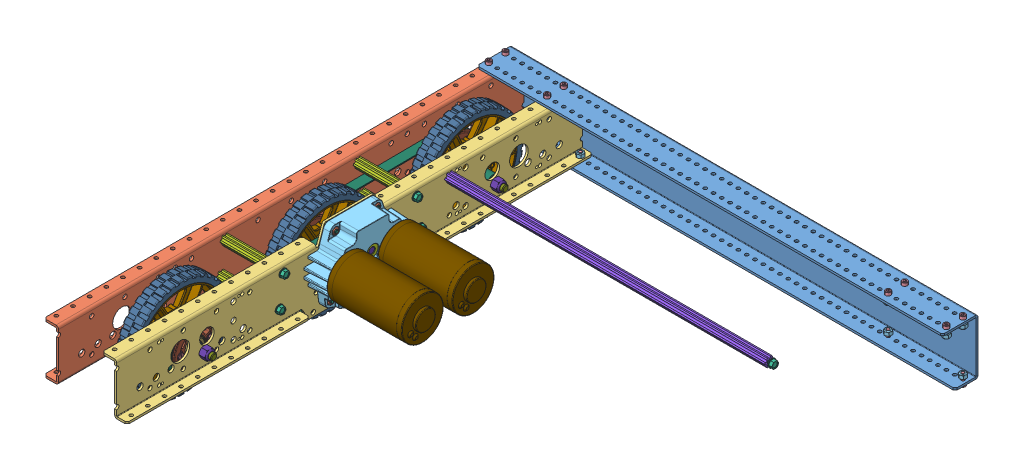
SolidWorks assembly AM14U4 Square Half, configuration Default. Lengths in mm.
Overall size (712.3 208.25 715.14).
150 component instances, 36 part files, 32 mates.
Components (placement in the parent):
- AM14U4 Square Frame Half-1: AM14U4 Square Frame Half [Default] at (318.96 74.5321 -359.8105) size (712.3 116.33 715.14)
  - am-xxxx AM14U4 End Plate Square-1: am-xxxx AM14U4 End Plate Square [Default] at (-787.4 -81.407 -3.175) x (1 0 0) z (0 -1 0) size (711.2 53.98 84.58)
  - am-xxxx AM14U4 Outside Plate Square-1: am-xxxx AM14U4 Outside Plate Square [DefaultSM-FLAT-PATTERN] at (-692.15 -77.216 762.762) x (0 0 -1) z (0 -1 0) size (711.2 22.23 77.72)
  - am-xxxx AM14U4 Inside Plate Square-1: am-xxxx AM14U4 Inside Plate Square [Default] at (-603.25 -77.216 762.762) x (0 0 -1) z (0 -1 0) size (711.2 38.1 116.33)
  - am-1002 and am-1042 10-32 x 0500 and Nylock Nut Assembly-2: am-1002 and am-1042 10-32 x 0500 and Nylock Nut Assembly [Default] at (-708.3821 -6.6363 35.2132) x (0 -1 0) z (0 0 1) size (17.53 13.8 13)
    - 10-32x0500_shcs-1: 10-32x0500_shcs [HX-SHCS 0.19-32x1.375x1-C] at (-11.4623 3.5321 3.6488) size (17.53 7.94 7.94)
    - 10-32 Nylock Nut 1-1: 10-32 Nylock Nut 1 [90631A411] at (-0.0323 3.5321 3.6488) x (0 0.381849 -0.924225) z (0 -0.924225 -0.381849) size (9.53 6.11 11)
  - am-1002 and am-1042 10-32 x 0500 and Nylock Nut Assembly-3: am-1002 and am-1042 10-32 x 0500 and Nylock Nut Assembly [Default] at (-708.3821 -6.6363 9.8132) x (0 -1 0) z (0 0 1) size (17.53 13.8 13)
    - 10-32x0500_shcs-1: 10-32x0500_shcs [HX-SHCS 0.19-32x1.375x1-C] at (-11.4623 3.5321 3.6488) size (17.53 7.94 7.94)
    - 10-32 Nylock Nut 1-1: 10-32 Nylock Nut 1 [90631A411] at (-0.0323 3.5321 3.6488) x (0 0.381849 -0.924225) z (0 -0.924225 -0.381849) size (9.53 6.11 11)
  - am-1002 and am-1042 10-32 x 0500 and Nylock Nut Assembly-7: am-1002 and am-1042 10-32 x 0500 and Nylock Nut Assembly [Default] at (-701.3179 -77.9457 9.8132) x (0 1 0) z (0 0 1) size (17.53 13.8 13)
    - 10-32x0500_shcs-1: 10-32x0500_shcs [HX-SHCS 0.19-32x1.375x1-C] at (-11.4623 3.5321 3.6488) size (17.53 7.94 7.94)
    - 10-32 Nylock Nut 1-1: 10-32 Nylock Nut 1 [90631A411] at (-0.0323 3.5321 3.6488) x (0 0.381849 -0.924225) z (0 -0.924225 -0.381849) size (9.53 6.11 11)
  - am-1002 and am-1042 10-32 x 0500 and Nylock Nut Assembly-8: am-1002 and am-1042 10-32 x 0500 and Nylock Nut Assembly [Default] at (-9.8821 -6.6363 9.8132) x (0 -1 0) z (0 0 1) size (17.53 13.8 13)
    - 10-32x0500_shcs-1: 10-32x0500_shcs [HX-SHCS 0.19-32x1.375x1-C] at (-11.4623 3.5321 3.6488) size (17.53 7.94 7.94)
    - 10-32 Nylock Nut 1-1: 10-32 Nylock Nut 1 [90631A411] at (-0.0323 3.5321 3.6488) x (0 0.381849 -0.924225) z (0 -0.924225 -0.381849) size (9.53 6.11 11)
  - am-1002 and am-1042 10-32 x 0500 and Nylock Nut Assembly-9: am-1002 and am-1042 10-32 x 0500 and Nylock Nut Assembly [Default] at (-9.8821 -6.6363 35.2132) x (0 -1 0) z (0 0 1) size (17.53 13.8 13)
    - 10-32x0500_shcs-1: 10-32x0500_shcs [HX-SHCS 0.19-32x1.375x1-C] at (-11.4623 3.5321 3.6488) size (17.53 7.94 7.94)
    - 10-32 Nylock Nut 1-1: 10-32 Nylock Nut 1 [90631A411] at (-0.0323 3.5321 3.6488) x (0 0.381849 -0.924225) z (0 -0.924225 -0.381849) size (9.53 6.11 11)
  - am-1002 and am-1042 10-32 x 0500 and Nylock Nut Assembly-10: am-1002 and am-1042 10-32 x 0500 and Nylock Nut Assembly [Default] at (-2.8179 -77.9457 9.8132) x (0 1 0) z (0 0 1) size (17.53 13.8 13)
    - 10-32x0500_shcs-1: 10-32x0500_shcs [HX-SHCS 0.19-32x1.375x1-C] at (-11.4623 3.5321 3.6488) size (17.53 7.94 7.94)
    - 10-32 Nylock Nut 1-1: 10-32 Nylock Nut 1 [90631A411] at (-0.0323 3.5321 3.6488) x (0 0.381849 -0.924225) z (0 -0.924225 -0.381849) size (9.53 6.11 11)
  - am-1002 and am-1042 10-32 x 0500 and Nylock Nut Assembly-11: am-1002 and am-1042 10-32 x 0500 and Nylock Nut Assembly [Default] at (-117.1179 -77.9457 9.8132) x (0 1 0) z (0 0 1) size (17.53 13.8 13)
    - 10-32x0500_shcs-1: 10-32x0500_shcs [HX-SHCS 0.19-32x1.375x1-C] at (-11.4623 3.5321 3.6488) size (17.53 7.94 7.94)
    - 10-32 Nylock Nut 1-1: 10-32 Nylock Nut 1 [90631A411] at (-0.0323 3.5321 3.6488) x (0 0.381849 -0.924225) z (0 -0.924225 -0.381849) size (9.53 6.11 11)
  - am-1002 and am-1042 10-32 x 0500 and Nylock Nut Assembly-12: am-1002 and am-1042 10-32 x 0500 and Nylock Nut Assembly [Default] at (-98.7821 -6.6363 35.2132) x (0 -1 0) z (0 0 1) size (17.53 13.8 13)
    - 10-32x0500_shcs-1: 10-32x0500_shcs [HX-SHCS 0.19-32x1.375x1-C] at (-11.4623 3.5321 3.6488) size (17.53 7.94 7.94)
    - 10-32 Nylock Nut 1-1: 10-32 Nylock Nut 1 [90631A411] at (-0.0323 3.5321 3.6488) x (0 0.381849 -0.924225) z (0 -0.924225 -0.381849) size (9.53 6.11 11)
  - am-1002 and am-1042 10-32 x 0500 and Nylock Nut Assembly-13: am-1002 and am-1042 10-32 x 0500 and Nylock Nut Assembly [Default] at (-98.7821 -6.6363 9.8132) x (0 -1 0) z (0 0 1) size (17.53 13.8 13)
    - 10-32x0500_shcs-1: 10-32x0500_shcs [HX-SHCS 0.19-32x1.375x1-C] at (-11.4623 3.5321 3.6488) size (17.53 7.94 7.94)
    - 10-32 Nylock Nut 1-1: 10-32 Nylock Nut 1 [90631A411] at (-0.0323 3.5321 3.6488) x (0 0.381849 -0.924225) z (0 -0.924225 -0.381849) size (9.53 6.11 11)
  - FHTS 0.25-20-0.75-1: FHTS 0.25-20-0.75 [FHTS 0.25-20-G-0.75-C] at (-692.15 -59.6687 248.8365) size (24.64 12.19 12.19)
  - FHTS 0.25-20-0.75-2: FHTS 0.25-20-0.75 [FHTS 0.25-20-G-0.75-C] at (-692.15 -14.986 254.762) size (24.64 12.19 12.19)
  - FHTS 0.25-20-0.75-3: FHTS 0.25-20-0.75 [FHTS 0.25-20-G-0.75-C] at (-692.15 -14.986 457.962) size (24.64 12.19 12.19)
  - FHTS 0.25-20-0.75-4: FHTS 0.25-20-0.75 [FHTS 0.25-20-G-0.75-C] at (-692.15 -59.6687 463.8875) size (24.64 12.19 12.19)
  - FHTS 0.25-20-0.75-5: FHTS 0.25-20-0.75 [FHTS 0.25-20-G-0.75-C] at (-600.075 -14.986 457.962) x (-1 0 0) z (0 0.924225 0.381849) size (24.64 12.19 12.19)
  - FHTS 0.25-20-0.75-6: FHTS 0.25-20-0.75 [FHTS 0.25-20-G-0.75-C] at (-600.075 -59.6687 463.8875) x (-1 0 0) z (0 0.924225 0.381849) size (24.64 12.19 12.19)
  - FHTS 0.25-20-0.75-7: FHTS 0.25-20-0.75 [FHTS 0.25-20-G-0.75-C] at (-600.075 -14.986 254.762) x (-1 0 0) z (0 0.924225 0.381849) size (24.64 12.19 12.19)
  - FHTS 0.25-20-0.75-8: FHTS 0.25-20-0.75 [FHTS 0.25-20-G-0.75-C] at (-600.075 -59.6687 248.8365) x (-1 0 0) z (0 0.924225 0.381849) size (24.64 12.19 12.19)
  - 3.375in Churro-1: 3.375in Churro [Default] at (-603.25 -14.986 254.762) x (0 0 1) z (-1 0 0) size (14.66 12.7 85.72)
  - 3.375in Churro-2: 3.375in Churro [Default] at (-606.425 -59.6687 248.8365) x (0 0 1) z (-1 0 0) size (14.66 12.7 85.72)
  - 3.375in Churro-3: 3.375in Churro [Default] at (-603.25 -14.986 457.962) x (0 0 1) z (-1 0 0) size (14.66 12.7 85.72)
  - 3.375in Churro-4: 3.375in Churro [Default] at (-603.25 -59.6687 463.8875) x (0 0 1) z (-1 0 0) size (14.66 12.7 85.72)
  - am-1002 and am-1042 10-32 x 0500 and Nylock Nut Assembly-14: am-1002 and am-1042 10-32 x 0500 and Nylock Nut Assembly [Default] at (-619.4821 -6.6363 9.8132) x (0 -1 0) z (0 0 1) size (17.53 13.8 13)
    - 10-32x0500_shcs-1: 10-32x0500_shcs [HX-SHCS 0.19-32x1.375x1-C] at (-11.4623 3.5321 3.6488) size (17.53 7.94 7.94)
    - 10-32 Nylock Nut 1-1: 10-32 Nylock Nut 1 [90631A411] at (-0.0323 3.5321 3.6488) x (0 0.381849 -0.924225) z (0 -0.924225 -0.381849) size (9.53 6.11 11)
  - am-1002 and am-1042 10-32 x 0500 and Nylock Nut Assembly-15: am-1002 and am-1042 10-32 x 0500 and Nylock Nut Assembly [Default] at (-619.4821 -6.6363 35.2132) x (0 -1 0) z (0 0 1) size (17.53 13.8 13)
    - 10-32x0500_shcs-1: 10-32x0500_shcs [HX-SHCS 0.19-32x1.375x1-C] at (-11.4623 3.5321 3.6488) size (17.53 7.94 7.94)
    - 10-32 Nylock Nut 1-1: 10-32 Nylock Nut 1 [90631A411] at (-0.0323 3.5321 3.6488) x (0 0.381849 -0.924225) z (0 -0.924225 -0.381849) size (9.53 6.11 11)
  - am-1002 and am-1042 10-32 x 0500 and Nylock Nut Assembly-16: am-1002 and am-1042 10-32 x 0500 and Nylock Nut Assembly [Default] at (-587.0179 -77.9457 9.8132) x (0 1 0) z (0 0 1) size (17.53 13.8 13)
    - 10-32x0500_shcs-1: 10-32x0500_shcs [HX-SHCS 0.19-32x1.375x1-C] at (-11.4623 3.5321 3.6488) size (17.53 7.94 7.94)
    - 10-32 Nylock Nut 1-1: 10-32 Nylock Nut 1 [90631A411] at (-0.0323 3.5321 3.6488) x (0 0.381849 -0.924225) z (0 -0.924225 -0.381849) size (9.53 6.11 11)
  - 19.25in Churro-1: 19.25in Churro [Default] at (-355.6 -14.986 203.962) x (0 0 1) z (-1 0 0) size (14.66 12.7 488.95)
  - FHTS 0.25-20-0.75-9: FHTS 0.25-20-0.75 [FHTS 0.25-20-G-0.75-C] at (-603.25 -14.986 203.962) size (24.64 12.19 12.19)
  - FHTS 0.25-20-0.75-10: FHTS 0.25-20-0.75 [FHTS 0.25-20-G-0.75-C] at (-107.95 -14.986 203.962) x (-1 0 0) z (0 -0.866025 -0.5) size (24.64 12.19 12.19)
- 6 HiGrip with bearings, pulleys and spacers-1: 6 HiGrip with bearings, pulleys and spacers [Default] at (-295.3634 -45.2429 -85.8734) x (-1 0 0) z (0 -0.111601 -0.993753) size (85.56 152.4 152.4)
  - 6 HiGrip Asm Rev II-1: 6 HiGrip Asm Rev II [Default] at (83.7987 67.439 110.9939) size (35.05 152.4 152.4)
    - 6 wheel Rev 4-1: 6 wheel Rev 4 [Default] at (-52.6446 9.4231 21.378) size (35.05 132.08 132.08)
    - 6 wheel tread II-1: 6 wheel tread II [Default] at (-65.3446 9.4231 21.378) x (0 0 -1) z (1 0 0) size (152.4 152.4 25.58)
  - 42 tooth HTD Pulley half 2014-1: 42 tooth HTD Pulley half 2014 [Default] at (47.6006 76.862 132.3719) x (1 0 0) z (0 -0.5 0.866025) size (13 74.23 74.23)
  - 42 tooth HTD Pulley half 2014-2: 42 tooth HTD Pulley half 2014 [Default] at (64.263 76.862 132.3719) x (-1 0 0) z (0 -0.499927 0.866067) size (13 74.23 74.23)
  - 1614Z Bearing-1: 1614Z Bearing [Default] at (62.612 76.862 132.3719) x (0 -0.157148 -0.987575) z (-1 0 0) size (28.57 28.57 9.53)
  - 10-24 Hex Washer Rolling x 1.25-1: 10-24 Hex Washer Rolling x 1.25 [93882A213] at (63.247 76.8605 108.5602) x (0 0 -1) z (1 0 0) size (10.52 10.52 35.59)
  - 10-24 Hex Washer Rolling x 1.25-2: 10-24 Hex Washer Rolling x 1.25 [93882A213] at (63.247 97.4833 120.4656) x (0 0 -1) z (1 0 0) size (10.52 10.52 35.59)
  - 10-24 Hex Washer Rolling x 1.25-3: 10-24 Hex Washer Rolling x 1.25 [93882A213] at (63.247 56.2398 144.2799) x (0 0 -1) z (1 0 0) size (10.52 10.52 35.59)
  - 10-24 Hex Washer Rolling x 1.25-4: 10-24 Hex Washer Rolling x 1.25 [93882A213] at (63.247 76.8625 156.1852) x (0 -0.95788 -0.287168) z (1 0 0) size (10.52 10.52 35.59)
  - 10-24 Hex Washer Rolling x 1.25-5: 10-24 Hex Washer Rolling x 1.25 [93882A213] at (63.247 97.4843 144.2781) x (0 -0.868976 0.494854) z (1 0 0) size (10.52 10.52 35.59)
  - 10-24 Hex Washer Rolling x 1.25-6: 10-24 Hex Washer Rolling x 1.25 [93882A213] at (63.247 56.2388 120.4674) x (0 -0.977348 -0.211637) z (1 0 0) size (10.52 10.52 35.59)
  - am-1306 spacer 0280 WashersUSA 13RS052001-1: am-1306 spacer 0280 WashersUSA 13RS052001 [Default] at (74.4865 76.862 132.3719) x (0 -0.35357 0.935408) z (-1 0 0) size (13.16 13.16 7.11)
  - 1614Z Bearing-2: 1614Z Bearing [Default] at (15.2791 76.862 132.3719) x (0 0.155433 -0.987846) z (-1 0 0) size (28.57 28.57 9.53)
  - am-1307 850 long 380 id-1: am-1307 850 long 380 id [Default] at (10.5166 76.862 132.3719) x (0 0.971418 -0.237374) z (0 0.237374 0.971418) size (19.05 21.59 19.05)
- 6 HiGrip with bearings, pulleys and spacers-2: 6 HiGrip with bearings, pulleys and spacers [Default] at (-358.7765 -60.4959 86.7273) size (85.56 152.4 152.4)
  - 6 HiGrip Asm Rev II-1: 6 HiGrip Asm Rev II [Default] at (83.7987 67.439 110.9939) size (35.05 152.4 152.4)
    - 6 wheel Rev 4-1: 6 wheel Rev 4 [Default] at (-52.6446 9.4231 21.378) size (35.05 132.08 132.08)
    - 6 wheel tread II-1: 6 wheel tread II [Default] at (-65.3446 9.4231 21.378) x (0 0 -1) z (1 0 0) size (152.4 152.4 25.58)
  - 42 tooth HTD Pulley half 2014-1: 42 tooth HTD Pulley half 2014 [Default] at (47.6006 76.862 132.3719) x (1 0 0) z (0 -0.5 0.866025) size (13 74.23 74.23)
  - 42 tooth HTD Pulley half 2014-2: 42 tooth HTD Pulley half 2014 [Default] at (64.263 76.862 132.3719) x (-1 0 0) z (0 -0.499927 0.866067) size (13 74.23 74.23)
  - 1614Z Bearing-1: 1614Z Bearing [Default] at (62.612 76.862 132.3719) x (0 -0.157148 -0.987575) z (-1 0 0) size (28.57 28.57 9.53)
  - 10-24 Hex Washer Rolling x 1.25-1: 10-24 Hex Washer Rolling x 1.25 [93882A213] at (63.247 76.8605 108.5602) x (0 0 -1) z (1 0 0) size (10.52 10.52 35.59)
  - 10-24 Hex Washer Rolling x 1.25-2: 10-24 Hex Washer Rolling x 1.25 [93882A213] at (63.247 97.4833 120.4656) x (0 0 -1) z (1 0 0) size (10.52 10.52 35.59)
  - 10-24 Hex Washer Rolling x 1.25-3: 10-24 Hex Washer Rolling x 1.25 [93882A213] at (63.247 56.2398 144.2799) x (0 0 -1) z (1 0 0) size (10.52 10.52 35.59)
  - 10-24 Hex Washer Rolling x 1.25-4: 10-24 Hex Washer Rolling x 1.25 [93882A213] at (63.247 76.8625 156.1852) x (0 -0.95788 -0.287168) z (1 0 0) size (10.52 10.52 35.59)
  - 10-24 Hex Washer Rolling x 1.25-5: 10-24 Hex Washer Rolling x 1.25 [93882A213] at (63.247 97.4843 144.2781) x (0 -0.868976 0.494854) z (1 0 0) size (10.52 10.52 35.59)
  - 10-24 Hex Washer Rolling x 1.25-6: 10-24 Hex Washer Rolling x 1.25 [93882A213] at (63.247 56.2388 120.4674) x (0 -0.977348 -0.211637) z (1 0 0) size (10.52 10.52 35.59)
  - am-1306 spacer 0280 WashersUSA 13RS052001-1: am-1306 spacer 0280 WashersUSA 13RS052001 [Default] at (74.4865 76.862 132.3719) x (0 -0.35357 0.935408) z (-1 0 0) size (13.16 13.16 7.11)
  - 1614Z Bearing-2: 1614Z Bearing [Default] at (15.2791 76.862 132.3719) x (0 0.155433 -0.987846) z (-1 0 0) size (28.57 28.57 9.53)
  - am-1307 850 long 380 id-1: am-1307 850 long 380 id [Default] at (10.5166 76.862 132.3719) x (0 0.971418 -0.237374) z (0 0.237374 0.971418) size (19.05 21.59 19.05)
- FR8ZZ Hex Bearing-1: FR8ZZ Hex Bearing [Default] at (-376.4183 14.5881 -3.4485) x (0 0 -1) z (1 0 0) size (31.12 31.12 7.93)
- am-2598_107 2016 KOP Toughbox Mini-1: am-2598_107 2016 KOP Toughbox Mini [Default] at (-331.6566 4.5181 87.6522) x (0 0.001296 0.999999) z (-1 0 0) size (140.05 121.81 142.29)
  - Toughbox d07-1: Toughbox d07 [Default] at (-88.5589 93.4503 -52.3959) x (-0.336928 0.94153 0) z (0.94153 0.336928 0) size (11 38.23 9.52)
  - Toughbox d05-1: Toughbox d05 [Default] at (-91.0349 50.9043 -67.5597) x (-0.336928 0.94153 0) z (0 0 -1) size (65.97 66.04 10.16)
  - FR6ZZ Bearing-1: FR6ZZ Bearing [Default] at (-96.247 60.278 -52.5991) x (-0.893862 0.448342 0) z (0 0 1) size (24.69 24.69 7.16)
  - 10-32 Nylock Nut-1: 10-32 Nylock Nut [Default] at (-129.8464 -8.0737 -56.3837) x (0.501678 0.865055 0) z (0 0 -1) size (10.18 11.01 7.1)
  - 10-32 Nylock Nut-2: 10-32 Nylock Nut [Default] at (-59.2462 80.7349 -56.3837) x (0.999999 -0.001296 0) z (0 0 -1) size (10.18 11.01 7.1)
  - 10-32 Nylock Nut-3: 10-32 Nylock Nut [Default] at (-122.7461 80.8172 -56.3837) x (0.500567 0.865698 0) z (0 0 -1) size (10.18 11.01 7.1)
  - 10-32 Nylock Nut-4: 10-32 Nylock Nut [Default] at (-52.3764 -8.1741 -56.3837) x (-0.501678 -0.865055 0) z (0 0 -1) size (10.18 11.01 7.1)
  - 5-16 washer-1: 5-16 washer [Default] at (-52.3162 38.3079 -77.7705) x (0.38418 -0.923258 0) z (0 0 -1) size (17.53 17.53 1.47)
  - 5-16 washer-2: 5-16 washer [Default] at (-52.3162 38.3079 -76.2973) x (0.897267 -0.441488 0) z (0 0 -1) size (17.53 17.53 1.47)
  - 5-16 washer-3: 5-16 washer [Default] at (-129.7861 38.4083 -77.7705) x (-0.990116 0.140253 0) z (0 0 1) size (17.53 17.53 1.47)
  - 5-16 washer-4: 5-16 washer [Default] at (-129.7861 38.4083 -79.2437) x (-0.681761 0.731575 0) z (0 0 1) size (17.53 17.53 1.47)
  - Toughbox d09-1: Toughbox d09 [Default] at (-52.3162 38.3079 -63.5973) x (0.910249 -0.414061 0) z (0 0 -1) size (20.03 20.32 12.7)
  - Toughbox d09-2: Toughbox d09 [Default] at (-129.7861 38.4083 -63.5973) x (0.075368 -0.997156 0) z (0 0 -1) size (20.03 20.32 12.7)
  - TM Housing-1: TM Housing [Default] at (-91.0876 10.1882 -86.3557) x (0.999999 -0.001296 0) z (0 0 1) size (139.9 118.55 41.54)
  - SHCS 10-32 x 0.625-1: SHCS 10-32 x 0.625 [Default] at (-52.2832 63.7078 -74.4685) x (-0.564778 -0.825243 0) z (-0.825243 0.564778 0) size (7.82 20.65 7.82)
  - SHCS 10-32 x 0.625-2: SHCS 10-32 x 0.625 [Default] at (-122.7461 80.8172 -42.5915) x (0.507484 -0.861661 0) z (-0.861661 -0.507484 0) size (7.82 20.65 7.82)
  - SHCS 10-32 x 0.625-3: SHCS 10-32 x 0.625 [Default] at (-52.3764 -8.1741 -42.5915) x (0.507484 -0.861661 0) z (-0.861661 -0.507484 0) size (7.82 20.65 7.82)
  - SHCS 10-32 x 0.625-4: SHCS 10-32 x 0.625 [Default] at (-129.8464 -8.0737 -42.5915) x (0.507484 -0.861661 0) z (-0.861661 -0.507484 0) size (7.82 20.65 7.82)
  - SHCS 10-32 x 0.625-5: SHCS 10-32 x 0.625 [Default] at (-59.2462 80.7349 -42.5915) x (0.740711 -0.671824 0) z (-0.671824 -0.740711 0) size (7.82 20.65 7.82)
  - SHCS 10-32 x 0.625-6: SHCS 10-32 x 0.625 [Default] at (-52.3491 12.9079 -74.4685) x (-0.564778 -0.825243 0) z (-0.825243 0.564778 0) size (7.82 20.65 7.82)
  - SHCS 10-32 x 0.625-7: SHCS 10-32 x 0.625 [Default] at (-129.7532 63.8083 -74.4685) x (-0.966277 -0.257503 0) z (-0.257503 0.966277 0) size (7.82 20.65 7.82)
  - SHCS 10-32 x 0.625-8: SHCS 10-32 x 0.625 [Default] at (-129.819 13.0083 -74.4685) x (-0.99652 0.083357 0) z (0.083357 0.99652 0) size (7.82 20.65 7.82)
  - R6ZZ Bearing-3: R6ZZ Bearing [Default] at (-91.0349 50.9043 -84.8317) x (0.958138 -0.286306 0) z (0 0 1) size (22.23 22.23 7.11)
  - R6ZZ Bearing-4: R6ZZ Bearing [Default] at (-91.0876 10.1882 -84.8317) x (-0.328282 -0.94458 0) z (0 0 1) size (22.23 22.23 7.11)
  - 8mm spring clip-1: 8mm spring clip [Default] at (-129.7861 38.4083 -63.5973) x (0 0 1) z (-1 0 0) size (1.09 14.83 14.83)
  - 8mm spring clip-2: 8mm spring clip [Default] at (-52.3162 38.3079 -63.5973) x (0 0 1) z (-1 0 0) size (1.09 14.83 14.83)
  - 500 E-klip-1: 500 E-klip [Default] at (-91.0876 10.1882 -64.4355) x (0.996411 -0.084651 0) z (0 0 1) size (19.07 20.96 1.27)
  - FR8ZZ Hex Bearing-1: FR8ZZ Hex Bearing [Default] at (-91.0876 10.1882 -44.6717) x (-0.5 0.866025 0) z (0 0 -1) size (31.12 31.12 7.93)
  - 16t 20dp 375h with teeth-1: 16t 20dp 375h with teeth [Default] at (-91.0349 50.9043 -67.5597) x (0 0 1) z (-0.983853 0.178977 0) size (15.19 22.57 22.57)
  - 48t 20dp 500h with teeth-1: 48t 20dp 500h with teeth [Default] at (-91.0876 10.1882 -63.1655) x (0 0 1) z (-1 0 0) size (10.21 63.42 63.42)
  - TB Output Shaft Hex L-Base 2-1: TB Output Shaft Hex L-Base 2 [Default] at (-52.7805 -6.4809 -52.3197) x (1 0 0) z (0 -1 0) size (14.66 142.29 12.7)
- 6 HiGrip with hub and double pulley-1: 6 HiGrip with hub and double pulley [Default] at (-295.2897 167.6569 -3.2676) x (-1 0 0) z (0 -0.865376 0.501122) size (81.42 152.4 152.4)
  - 6 HiGrip Asm Rev II-1: 6 HiGrip Asm Rev II [Default] at (83.7987 67.439 110.9939) size (35.05 152.4 152.4)
    - 6 wheel Rev 4-1: 6 wheel Rev 4 [Default] at (-52.6446 9.4231 21.378) size (35.05 132.08 132.08)
    - 6 wheel tread II-1: 6 wheel tread II [Default] at (-65.3446 9.4231 21.378) x (0 0 -1) z (1 0 0) size (152.4 152.4 25.58)
  - 42 tooth HTD Pulley half 2014-1: 42 tooth HTD Pulley half 2014 [Default] at (47.6006 76.862 132.3719) x (1 0 0) z (0 -0.5 0.866025) size (13 74.23 74.23)
  - 42 tooth HTD Pulley half 2014-2: 42 tooth HTD Pulley half 2014 [Default] at (64.263 76.862 132.3719) x (-1 0 0) z (0 -0.499927 0.866067) size (13 74.23 74.23)
  - 10-24 Hex Washer Rolling x 1.25-1: 10-24 Hex Washer Rolling x 1.25 [93882A213] at (63.247 76.8605 108.5602) x (0 0 -1) z (1 0 0) size (10.52 10.52 35.59)
  - 10-24 Hex Washer Rolling x 1.25-2: 10-24 Hex Washer Rolling x 1.25 [93882A213] at (63.247 97.4833 120.4656) x (0 0 -1) z (1 0 0) size (10.52 10.52 35.59)
  - 10-24 Hex Washer Rolling x 1.25-3: 10-24 Hex Washer Rolling x 1.25 [93882A213] at (63.247 56.2398 144.2799) x (0 0 -1) z (1 0 0) size (10.52 10.52 35.59)
  - 10-24 Hex Washer Rolling x 1.25-4: 10-24 Hex Washer Rolling x 1.25 [93882A213] at (63.247 76.8625 156.1852) x (0 -0.95788 -0.287168) z (1 0 0) size (10.52 10.52 35.59)
  - 10-24 Hex Washer Rolling x 1.25-5: 10-24 Hex Washer Rolling x 1.25 [93882A213] at (63.247 97.4843 144.2781) x (0 -0.868976 0.494854) z (1 0 0) size (10.52 10.52 35.59)
  - 10-24 Hex Washer Rolling x 1.25-6: 10-24 Hex Washer Rolling x 1.25 [93882A213] at (63.247 56.2388 120.4674) x (0 -0.748729 -0.662876) z (1 0 0) size (10.52 10.52 35.59)
  - 42 tooth HTD Pulley half 2014-3: 42 tooth HTD Pulley half 2014 [Default] at (-1.9548 76.8628 132.3714) x (1 0 0) z (0 -1 -0.000063) size (13 74.23 74.23)
  - 42 tooth HTD Pulley half 2014-4: 42 tooth HTD Pulley half 2014 [Default] at (14.7076 76.8628 132.3714) x (-1 0 0) z (0 -1 0.000021) size (13 74.23 74.23)
  - 500EX Hex Hub-1: 500EX Hex Hub [Default] at (-8.3048 76.8628 132.3714) x (0 -0.866025 -0.5) z (0 -0.5 0.866025) size (55.37 25.4 51.33)
  - 10-24 Hex Washer Rolling x 1.25-7: 10-24 Hex Washer Rolling x 1.25 [93882A213] at (-5.2568 97.485 120.4652) x (0 0 1) z (-1 0 0) size (10.52 10.52 35.59)
  - 10-24 Hex Washer Rolling x 1.25-8: 10-24 Hex Washer Rolling x 1.25 [93882A213] at (-5.2568 76.8628 108.5589) x (0 0 1) z (-1 0 0) size (10.52 10.52 35.59)
  - 10-24 Hex Washer Rolling x 1.25-9: 10-24 Hex Washer Rolling x 1.25 [93882A213] at (-5.2568 56.2406 120.4652) x (0 0 1) z (-1 0 0) size (10.52 10.52 35.59)
  - 10-24 Hex Washer Rolling x 1.25-10: 10-24 Hex Washer Rolling x 1.25 [93882A213] at (-5.2568 97.485 144.2777) x (0 -0.99374 -0.111715) z (-1 0 0) size (10.52 10.52 35.59)
  - 10-24 Hex Washer Rolling x 1.25-11: 10-24 Hex Washer Rolling x 1.25 [93882A213] at (-5.2568 56.2406 144.2777) x (0 -0.138911 0.990305) z (-1 0 0) size (10.52 10.52 35.59)
  - 10-24 Hex Washer Rolling x 1.25-12: 10-24 Hex Washer Rolling x 1.25 [93882A213] at (-5.2568 76.8628 156.1839) x (0 -0.98811 -0.15375) z (-1 0 0) size (10.52 10.52 35.59)
  - am-1305 500 Hex Spacer-1: am-1305 500 Hex Spacer [Default] at (57.8495 76.862 132.3719) x (0 -0.866025 -0.5) z (0 -0.5 0.866025) size (28.55 14.48 28.55)
- 655-5M-15 v2-1: 655-5M-15 v2 [Default] at (-357.8903 14.5881 -3.4485) x (0 0.007989 -0.999968) z (0 -0.999968 -0.007989) size (295.63 15 73.08)
- 655-5M-15 v2-2: 655-5M-15 v2 [Default] at (-309.9973 14.5881 -3.4485) x (0 0.007989 0.999968) z (0 0.999968 -0.007989) size (295.63 15 73.08)
- 375-16 x 4.25 Hex Bolt-1: 375-16 x 4.25 Hex Bolt [HFBOLT 0.375-16x2.5x1-C] at (-379.3622 16.3661 -225.9962) size (114.12 16.48 14.27)
- 375-16 x 4.25 Hex Bolt-2: 375-16 x 4.25 Hex Bolt [HFBOLT 0.375-16x2.5x1-C] at (-379.3622 16.3661 219.0992) size (114.12 16.48 14.27)
- 3-8-16 NyLock Nut - Mcm 95615A140-1: 3-8-16 NyLock Nut - Mcm 95615A140 [95615A140] at (-281.115 16.3661 -225.9962) x (0 -1 0) z (0 0 1) size (14.29 12 16.5)
- 3-8-16 NyLock Nut - Mcm 95615A140-2: 3-8-16 NyLock Nut - Mcm 95615A140 [95615A140] at (-281.115 16.3661 219.0992) x (0 -1 0) z (0 0 1) size (14.29 12 16.5)
- CIM Motor SW-1: CIM Motor SW [Default] at (-226.251 78.3181 -151.4797) x (0 -1 0) z (-1 0 0) size (64.01 64.01 154.93)
- CIM Motor SW-2: CIM Motor SW [Default] at (-226.251 78.3181 -74.0097) x (0 -1 0) z (-1 0 0) size (64.01 64.01 154.93)
Mates (geometry in assembly coordinates):
- Coincident1: coincident: plane of AM14U4 Square Frame Half-1/am-xxxx AM14U4 Inside Plate Square-1 through (-284.29 67.1661 402.9515) normal (-1 0 0); plane of 6 HiGrip with bearings, pulleys and spacers-2/am-1306 spacer 0280 WashersUSA 13RS052001-1 through (-284.29 16.3661 219.0992) normal (1 0 0)
- Concentric1: concentric: circle of AM14U4 Square Frame Half-1/am-xxxx AM14U4 Inside Plate Square-1; cylinder of 6 HiGrip with bearings, pulleys and spacers-2/am-1306 spacer 0280 WashersUSA 13RS052001-1 through (-291.402 16.3661 219.0992) axis (1 0 0) radius 6.5786
- Coincident2: coincident: plane of AM14U4 Square Frame Half-1/am-xxxx AM14U4 Inside Plate Square-1 through (-284.29 67.1661 402.9515) normal (-1 0 0); plane of 6 HiGrip with bearings, pulleys and spacers-1/am-1307 850 long 380 id-1 through (-284.29 16.3661 -225.9962) normal (1 0 0)
- Concentric2: concentric: circle of AM14U4 Square Frame Half-1/am-xxxx AM14U4 Inside Plate Square-1; cylinder of 6 HiGrip with bearings, pulleys and spacers-1/am-1307 850 long 380 id-1 through (-284.29 16.3661 -225.9962) axis (-1 0 0) radius 9.525
- Concentric31: concentric: cylinder of AM14U4 Square Frame Half-1/am-xxxx AM14U4 Outside Plate Square-1 through (-373.19 14.5881 -3.4485) axis (1 0 0) radius 14.2875; cylinder of FR8ZZ Hex Bearing-1 through (-368.491 14.5881 -3.4485) axis (-1 0 0) radius 13.97
- Coincident31: coincident: plane of AM14U4 Square Frame Half-1/am-xxxx AM14U4 Outside Plate Square-1 through (-370.015 67.1661 402.9515) normal (1 0 0); plane of FR8ZZ Hex Bearing-1 through (-370.015 14.5881 -17.4185) normal (-1 0 0)
- Concentric4: concentric: cylinder of AM14U4 Square Frame Half-1/am-xxxx AM14U4 Inside Plate Square-1 through (-284.29 14.5881 -3.4485) axis (1 0 0) radius 14.2875; cylinder of am-2598_107 2016 KOP Toughbox Mini-1/FR8ZZ Hex Bearing-1 through (-279.0576 14.5881 -3.4485) axis (-1 0 0) radius 14.2875
- Parallel1: parallel: plane of AM14U4 Square Frame Half-1/am-xxxx AM14U4 Inside Plate Square-1 through (-281.115 94.5981 -51.0735) normal (0 1 0); line of am-2598_107 2016 KOP Toughbox Mini-1/TM Housing-1 through (-280.5893 94.1554 -35.1985) axis (0 0 1)
- Coincident5: coincident: plane of AM14U4 Square Frame Half-1/am-xxxx AM14U4 Inside Plate Square-1 through (-281.115 67.1661 402.9515) normal (1 0 0); plane of am-2598_107 2016 KOP Toughbox Mini-1/TM Housing-1 through (-281.115 14.5881 -3.4485) normal (-1 0 0)
- Concentric5: concentric: cylinder of am-2598_107 2016 KOP Toughbox Mini-1/FR8ZZ Hex Bearing-1 through (-279.0576 14.5881 -3.4485) axis (-1 0 0) radius 14.2875; circle of 6 HiGrip with hub and double pulley-1/500EX Hex Hub-1
- Parallel2: parallel: plane of am-2598_107 2016 KOP Toughbox Mini-1/TB Output Shaft Hex L-Base 2-1 through (-253.937 20.9429 0.2094) normal (0 0.999999 -0.001296); plane of 6 HiGrip with hub and double pulley-1/500EX Hex Hub-1 through (-286.9849 8.2207 -7.1138) normal (0 0.999999 -0.001296)
- Coincident7: coincident: plane of am-2598_107 2016 KOP Toughbox Mini-1/FR8ZZ Hex Bearing-1 through (-286.9849 14.5881 -3.4485) normal (-1 0 0); plane of 6 HiGrip with hub and double pulley-1/500EX Hex Hub-1 through (-286.9849 14.5881 -3.4485) normal (1 0 0)
- Concentric6: concentric: circle of AM14U4 Square Frame Half-1/am-xxxx AM14U4 Outside Plate Square-1; cylinder of 655-5M-15 v2-2 through (-294.9973 16.3661 219.0992) axis (-1 0 0) radius 35.0139
- Concentric7: concentric: cylinder of FR8ZZ Hex Bearing-1 through (-368.491 14.5881 -3.4485) axis (-1 0 0) radius 14.2875; cylinder of 655-5M-15 v2-2 through (-294.9973 14.5881 -3.4485) axis (-1 0 0) radius 36.5379
- Concentric8: concentric: cylinder of AM14U4 Square Frame Half-1/am-xxxx AM14U4 Outside Plate Square-1 through (-481.141 16.3661 -225.9962) axis (1 0 0) radius 4.826; cylinder of 655-5M-15 v2-1 through (-342.8903 16.3661 -225.9962) axis (-1 0 0) radius 35.0139
- Concentric9: concentric: circle of AM14U4 Square Frame Half-1/am-xxxx AM14U4 Outside Plate Square-1; cylinder of 655-5M-15 v2-1 through (-342.8903 14.5881 -3.4485) axis (-1 0 0) radius 36.5379
- Coincident10: coincident: plane of 6 HiGrip with hub and double pulley-1/42 tooth HTD Pulley half 2014-1 through (-342.8903 14.5882 -3.4477) normal (-1 0 0); plane of 655-5M-15 v2-1 through (-342.8903 14.5881 -3.4485) normal (1 0 0)
- Coincident11: coincident: plane of 6 HiGrip with hub and double pulley-1/42 tooth HTD Pulley half 2014-4 through (-309.9973 14.5881 -3.4485) normal (1 0 0); plane of 655-5M-15 v2-2 through (-309.9973 14.5881 -3.4485) normal (-1 0 0)
- Concentric101: concentric: cylinder of AM14U4 Square Frame Half-1/am-xxxx AM14U4 Outside Plate Square-1 through (-481.141 16.3661 -225.9962) axis (1 0 0) radius 4.826; cylinder of 375-16 x 4.25 Hex Bolt-1 through (-379.3622 16.3661 -225.9962) axis (-1 0 0) radius 7.1374
- Coincident121: coincident: plane of AM14U4 Square Frame Half-1/am-xxxx AM14U4 Outside Plate Square-1 through (-373.19 67.1661 402.9515) normal (-1 0 0); plane of 375-16 x 4.25 Hex Bolt-1 through (-373.19 24.6077 -225.9962) normal (1 0 0)
- Concentric111: concentric: cylinder of AM14U4 Square Frame Half-1/am-xxxx AM14U4 Outside Plate Square-1 through (-481.141 16.3661 219.0992) axis (1 0 0) radius 4.826; cylinder of 375-16 x 4.25 Hex Bolt-2 through (-379.3622 16.3661 219.0992) axis (-1 0 0) radius 7.1374
- Coincident131: coincident: plane of AM14U4 Square Frame Half-1/am-xxxx AM14U4 Outside Plate Square-1 through (-373.19 67.1661 402.9515) normal (-1 0 0); plane of 375-16 x 4.25 Hex Bolt-2 through (-373.19 24.6077 219.0992) normal (1 0 0)
- Coincident14: coincident: plane of AM14U4 Square Frame Half-1/am-xxxx AM14U4 Inside Plate Square-1 through (-281.115 67.1661 402.9515) normal (1 0 0); plane of 3-8-16 NyLock Nut - Mcm 95615A140-1 through (-281.115 23.5099 -238.3696) normal (-1 0 0)
- Coincident15: coincident: plane of AM14U4 Square Frame Half-1/am-xxxx AM14U4 Inside Plate Square-1 through (-281.115 67.1661 402.9515) normal (1 0 0); plane of 3-8-16 NyLock Nut - Mcm 95615A140-2 through (-281.115 23.5099 206.7258) normal (-1 0 0)
- Concentric12: concentric: cylinder of 375-16 x 4.25 Hex Bolt-2 through (-379.3622 16.3661 219.0992) axis (-1 0 0) radius 4.7625; cylinder of 3-8-16 NyLock Nut - Mcm 95615A140-2 through (-271.4476 16.3661 219.0992) axis (-1 0 0) radius 4.0291
- Concentric13: concentric: cylinder of 375-16 x 4.25 Hex Bolt-1 through (-379.3622 16.3661 -225.9962) axis (-1 0 0) radius 4.7625; cylinder of 3-8-16 NyLock Nut - Mcm 95615A140-1 through (-271.4476 16.3661 -225.9962) axis (-1 0 0) radius 4.0291
- Coincident16: coincident: plane of CIM Motor SW-1 through (-245.301 42.7581 -42.1835) normal (-1 0 0); plane of CIM Motor SW-2 through (-245.301 42.7581 35.2865) normal (-1 0 0)
- Concentric14: concentric: cylinder of am-2598_107 2016 KOP Toughbox Mini-1/TM Housing-1 through (-281.115 42.7581 -42.1835) axis (-1 0 0) radius 10.414; cylinder of CIM Motor SW-1 through (-237.0714 42.7581 -42.1835) axis (1 0 0) radius 32.004
- Concentric15: concentric: cylinder of am-2598_107 2016 KOP Toughbox Mini-1/TM Housing-1 through (-281.115 42.7581 35.2865) axis (-1 0 0) radius 10.414; cylinder of CIM Motor SW-2 through (-237.0714 42.7581 35.2865) axis (1 0 0) radius 32.004
- Concentric16: concentric: cylinder of am-2598_107 2016 KOP Toughbox Mini-1/SHCS 10-32 x 0.625-6 through (-236.538 17.3581 35.2865) axis (-1 0 0) radius 2.3876; circle of CIM Motor SW-2
- Concentric17: concentric: cylinder of am-2598_107 2016 KOP Toughbox Mini-1/SHCS 10-32 x 0.625-8 through (-236.538 17.3581 -42.1835) axis (-1 0 0) radius 2.3876; cylinder of CIM Motor SW-1 through (-245.301 17.3581 -42.1835) axis (-1 0 0) radius 2.0193
- Coincident17: coincident: plane of am-2598_107 2016 KOP Toughbox Mini-1/TM Housing-1 through (-245.301 14.5881 -3.4485) normal (1 0 0); plane of CIM Motor SW-1 through (-245.301 42.7581 -42.1835) normal (-1 0 0)
